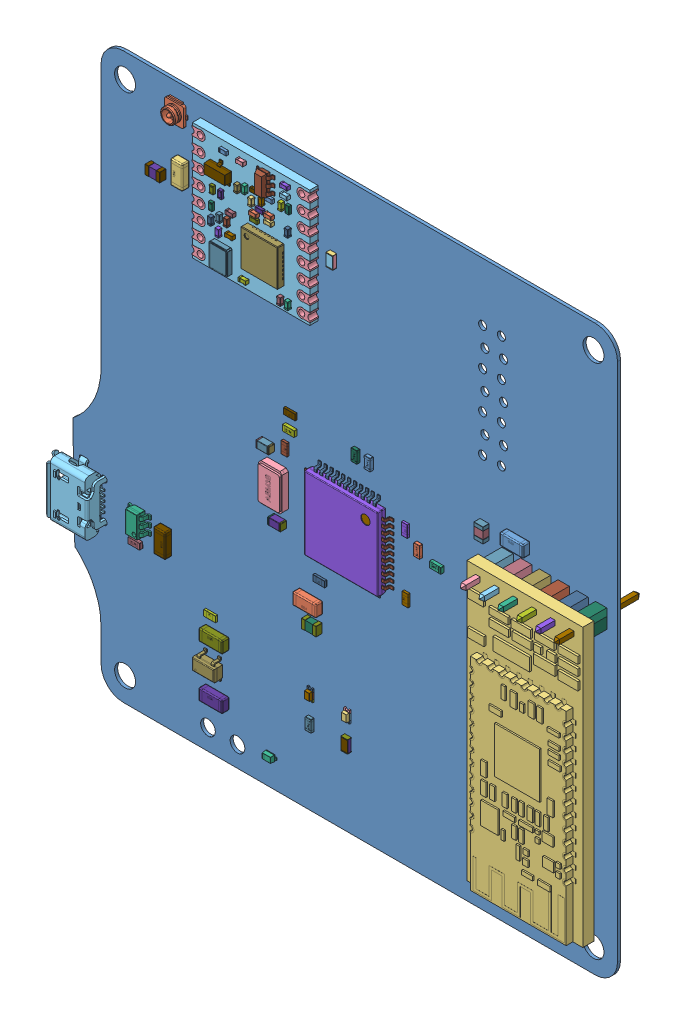
SolidWorks assembly Печатная плата Peggy Receiver, configuration Default. Lengths in mm. (continued)
Components (placement in the parent): (continued)
- Печатная плата Peggy Receiver(2)^Печатная плата Peggy Receiver-2: Печатная плата Peggy Receiver(2)^Печатная плата Peggy Receiver [Default] at origin size (75.31 78.06 11.44) (virtual) (continued)
  - DD1^Печатная плата Peggy Receiver(2)_Печатная плата Peggy Receiver-2: DD1^Печатная плата Peggy Receiver(2)_Печатная плата Peggy Receiver [Default] at origin size (16 15.9 2.23) (virtual) (continued)
    - User Library-RFM96W^DD1_Печатная плата Peggy Receiver(2)_Печатная плата Peggy Receiver-1: User Library-RFM96W^DD1_Печатная плата Peggy Receiver(2)_Печатная плата Peggy Receiver [Default] at (17.298 57.975 1.15) x (1 0 0) z (0 0 1) size (16 15.9 2.23) (virtual) (continued)
      - Designator8^User Library-RFM96W_DD1_Печатная плата Peggy Receiver(2)_Печатная плата Peggy Receiver-1: Designator8^User Library-RFM96W_DD1_Печатная плата Peggy Receiver(2)_Печатная плата Peggy Receiver [Default] at origin size (1 0.5 0.5) (virtual)
        - Cap0402^Designator8_User Library-RFM96W_DD1_Печатная плата Peggy Receiver(2)_Печатная плата Peggy Receiver-1: Cap0402^Designator8_User Library-RFM96W_DD1_Печатная плата Peggy Receiver(2)_Печатная плата Peggy Receiver [Default] at (5.4 5.45 0) x (1 0 0) z (0 -1 0) size (1 0.5 0.5) (virtual)
      - Designator9^User Library-RFM96W_DD1_Печатная плата Peggy Receiver(2)_Печатная плата Peggy Receiver-1: Designator9^User Library-RFM96W_DD1_Печатная плата Peggy Receiver(2)_Печатная плата Peggy Receiver [Default] at origin size (0.5 1 0.5) (virtual)
        - Cap0402^Designator9_User Library-RFM96W_DD1_Печатная плата Peggy Receiver(2)_Печатная плата Peggy Receiver-1: Cap0402^Designator9_User Library-RFM96W_DD1_Печатная плата Peggy Receiver(2)_Печатная плата Peggy Receiver [Default] at (2.8 5.98 0) x (0 -1 0) z (-1 0 0) size (1 0.5 0.5) (virtual)
      - Designator10^User Library-RFM96W_DD1_Печатная плата Peggy Receiver(2)_Печатная плата Peggy Receiver-1: Designator10^User Library-RFM96W_DD1_Печатная плата Peggy Receiver(2)_Печатная плата Peggy Receiver [Default] at origin size (0.5 1 0.5) (virtual)
        - Cap0402^Designator10_User Library-RFM96W_DD1_Печатная плата Peggy Receiver(2)_Печатная плата Peggy Receiver-1: Cap0402^Designator10_User Library-RFM96W_DD1_Печатная плата Peggy Receiver(2)_Печатная плата Peggy Receiver [Default] at (4.953 6.858 0) x (0 -1 0) z (-1 0 0) size (1 0.5 0.5) (virtual)
      - Designator11^User Library-RFM96W_DD1_Печатная плата Peggy Receiver(2)_Печатная плата Peggy Receiver-1: Designator11^User Library-RFM96W_DD1_Печатная плата Peggy Receiver(2)_Печатная плата Peggy Receiver [Default] at origin size (0.5 1 0.5) (virtual)
        - Cap0402^Designator11_User Library-RFM96W_DD1_Печатная плата Peggy Receiver(2)_Печатная плата Peggy Receiver-1: Cap0402^Designator11_User Library-RFM96W_DD1_Печатная плата Peggy Receiver(2)_Печатная плата Peggy Receiver [Default] at (6.35 11.557 0) x (0 1 0) z (1 0 0) size (1 0.5 0.5) (virtual)
      - Designator12^User Library-RFM96W_DD1_Печатная плата Peggy Receiver(2)_Печатная плата Peggy Receiver-1: Designator12^User Library-RFM96W_DD1_Печатная плата Peggy Receiver(2)_Печатная плата Peggy Receiver [Default] at origin size (1 0.5 0.5) (virtual)
        - Cap0402^Designator12_User Library-RFM96W_DD1_Печатная плата Peggy Receiver(2)_Печатная плата Peggy Receiver-1: Cap0402^Designator12_User Library-RFM96W_DD1_Печатная плата Peggy Receiver(2)_Печатная плата Peggy Receiver [Default] at (5.461 8.128 0) x (1 0 0) z (0 -1 0) size (1 0.5 0.5) (virtual)
      - Designator13^User Library-RFM96W_DD1_Печатная плата Peggy Receiver(2)_Печатная плата Peggy Receiver-1: Designator13^User Library-RFM96W_DD1_Печатная плата Peggy Receiver(2)_Печатная плата Peggy Receiver [Default] at origin size (0.5 1 0.5) (virtual)
        - Cap0402^Designator13_User Library-RFM96W_DD1_Печатная плата Peggy Receiver(2)_Печатная плата Peggy Receiver-1: Cap0402^Designator13_User Library-RFM96W_DD1_Печатная плата Peggy Receiver(2)_Печатная плата Peggy Receiver [Default] at (3.937 6.858 0) x (0 1 0) z (1 0 0) size (1 0.5 0.5) (virtual)
      - Designator15^User Library-RFM96W_DD1_Печатная плата Peggy Receiver(2)_Печатная плата Peggy Receiver-1: Designator15^User Library-RFM96W_DD1_Печатная плата Peggy Receiver(2)_Печатная плата Peggy Receiver [Default] at origin size (0.52 1.02 0.37) (virtual)
        - SW3dPS-inductor_0402_white^Designator15_User Library-RFM96W_DD1_Печатная плата Peggy Receiver(2)_Печатная плата Peggy Receiver-1: SW3dPS-inductor_0402_white^Designator15_User Library-RFM96W_DD1_Печатная плата Peggy Receiver(2)_Печатная плата Peggy Receiver [Default] at (13.208 12.446 0) x (1 0 0) z (0 -1 0) size (0.52 0.37 1.02) (virtual)
      - Designator17^User Library-RFM96W_DD1_Печатная плата Peggy Receiver(2)_Печатная плата Peggy Receiver-1: Designator17^User Library-RFM96W_DD1_Печатная плата Peggy Receiver(2)_Печатная плата Peggy Receiver [Default] at origin size (1.02 0.52 0.37) (virtual)
        - SW3dPS-inductor_0402_white^Designator17_User Library-RFM96W_DD1_Печатная плата Peggy Receiver(2)_Печатная плата Peggy Receiver-1: SW3dPS-inductor_0402_white^Designator17_User Library-RFM96W_DD1_Печатная плата Peggy Receiver(2)_Печатная плата Peggy Receiver [Default] at (8.636 8.89 0) x (0 1 0) z (1 0 0) size (0.52 0.37 1.02) (virtual)
      - Designator18^User Library-RFM96W_DD1_Печатная плата Peggy Receiver(2)_Печатная плата Peggy Receiver-1: Designator18^User Library-RFM96W_DD1_Печатная плата Peggy Receiver(2)_Печатная плата Peggy Receiver [Default] at origin size (1.02 0.52 0.37) (virtual)
        - SW3dPS-inductor_0402_white^Designator18_User Library-RFM96W_DD1_Печатная плата Peggy Receiver(2)_Печатная плата Peggy Receiver-1: SW3dPS-inductor_0402_white^Designator18_User Library-RFM96W_DD1_Печатная плата Peggy Receiver(2)_Печатная плата Peggy Receiver [Default] at (9.398 10.414 0) x (0 1 0) z (1 0 0) size (0.52 0.37 1.02) (virtual)
      - Designator19^User Library-RFM96W_DD1_Печатная плата Peggy Receiver(2)_Печатная плата Peggy Receiver-1: Designator19^User Library-RFM96W_DD1_Печатная плата Peggy Receiver(2)_Печатная плата Peggy Receiver [Default] at origin size (1.02 0.52 0.37) (virtual)
        - SW3dPS-inductor_0402_white^Designator19_User Library-RFM96W_DD1_Печатная плата Peggy Receiver(2)_Печатная плата Peggy Receiver-1: SW3dPS-inductor_0402_white^Designator19_User Library-RFM96W_DD1_Печатная плата Peggy Receiver(2)_Печатная плата Peggy Receiver [Default] at (8.636 12.319 0) x (0 1 0) z (1 0 0) size (0.52 0.37 1.02) (virtual)
      - Designator20^User Library-RFM96W_DD1_Печатная плата Peggy Receiver(2)_Печатная плата Peggy Receiver-1: Designator20^User Library-RFM96W_DD1_Печатная плата Peggy Receiver(2)_Печатная плата Peggy Receiver [Default] at origin size (1.02 0.52 0.37) (virtual)
        - SW3dPS-inductor_0402_white^Designator20_User Library-RFM96W_DD1_Печатная плата Peggy Receiver(2)_Печатная плата Peggy Receiver-1: SW3dPS-inductor_0402_white^Designator20_User Library-RFM96W_DD1_Печатная плата Peggy Receiver(2)_Печатная плата Peggy Receiver [Default] at (10.668 12.319 0) x (0 1 0) z (1 0 0) size (0.52 0.37 1.02) (virtual)
      - Designator21^User Library-RFM96W_DD1_Печатная плата Peggy Receiver(2)_Печатная плата Peggy Receiver-1: Designator21^User Library-RFM96W_DD1_Печатная плата Peggy Receiver(2)_Печатная плата Peggy Receiver [Default] at origin size (1 0.5 0.5) (virtual)
        - Cap0402^Designator21_User Library-RFM96W_DD1_Печатная плата Peggy Receiver(2)_Печатная плата Peggy Receiver-1: Cap0402^Designator21_User Library-RFM96W_DD1_Печатная плата Peggy Receiver(2)_Печатная плата Peggy Receiver [Default] at (10.668 10.414 0) x (-1 0 0) z (0 1 0) size (1 0.5 0.5) (virtual)
      - Designator22^User Library-RFM96W_DD1_Печатная плата Peggy Receiver(2)_Печатная плата Peggy Receiver-1: Designator22^User Library-RFM96W_DD1_Печатная плата Peggy Receiver(2)_Печатная плата Peggy Receiver [Default] at origin size (0.5 1 0.5) (virtual)
        - Cap0402^Designator22_User Library-RFM96W_DD1_Печатная плата Peggy Receiver(2)_Печатная плата Peggy Receiver-1: Cap0402^Designator22_User Library-RFM96W_DD1_Печатная плата Peggy Receiver(2)_Печатная плата Peggy Receiver [Default] at (8.255 10.922 0) x (0 1 0) z (1 0 0) size (1 0.5 0.5) (virtual)
      - Designator23^User Library-RFM96W_DD1_Печатная плата Peggy Receiver(2)_Печатная плата Peggy Receiver-1: Designator23^User Library-RFM96W_DD1_Печатная плата Peggy Receiver(2)_Печатная плата Peggy Receiver [Default] at origin size (1 0.5 0.5) (virtual)
        - Cap0402^Designator23_User Library-RFM96W_DD1_Печатная плата Peggy Receiver(2)_Печатная плата Peggy Receiver-1: Cap0402^Designator23_User Library-RFM96W_DD1_Печатная плата Peggy Receiver(2)_Печатная плата Peggy Receiver [Default] at (6.858 14.859 0) x (-1 0 0) z (0 1 0) size (1 0.5 0.5) (virtual)
      - Designator24^User Library-RFM96W_DD1_Печатная плата Peggy Receiver(2)_Печатная плата Peggy Receiver-1: Designator24^User Library-RFM96W_DD1_Печатная плата Peggy Receiver(2)_Печатная плата Peggy Receiver [Default] at origin size (1 0.5 0.5) (virtual)
        - Cap0402^Designator24_User Library-RFM96W_DD1_Печатная плата Peggy Receiver(2)_Печатная плата Peggy Receiver-1: Cap0402^Designator24_User Library-RFM96W_DD1_Печатная плата Peggy Receiver(2)_Печатная плата Peggy Receiver [Default] at (12.827 13.843 0) x (-1 0 0) z (0 1 0) size (1 0.5 0.5) (virtual)
      - Designator25^User Library-RFM96W_DD1_Печатная плата Peggy Receiver(2)_Печатная плата Peggy Receiver-1: Designator25^User Library-RFM96W_DD1_Печатная плата Peggy Receiver(2)_Печатная плата Peggy Receiver [Default] at origin size (0.5 1 0.5) (virtual)
        - Cap0402^Designator25_User Library-RFM96W_DD1_Печатная плата Peggy Receiver(2)_Печатная плата Peggy Receiver-1: Cap0402^Designator25_User Library-RFM96W_DD1_Печатная плата Peggy Receiver(2)_Печатная плата Peggy Receiver [Default] at (7.366 11.938 0) x (0 -1 0) z (-1 0 0) size (1 0.5 0.5) (virtual)
      - Designator26^User Library-RFM96W_DD1_Печатная плата Peggy Receiver(2)_Печатная плата Peggy Receiver-1: Designator26^User Library-RFM96W_DD1_Печатная плата Peggy Receiver(2)_Печатная плата Peggy Receiver [Default] at origin size (0.5 1 0.5) (virtual)
        - Cap0402^Designator26_User Library-RFM96W_DD1_Печатная плата Peggy Receiver(2)_Печатная плата Peggy Receiver-1: Cap0402^Designator26_User Library-RFM96W_DD1_Печатная плата Peggy Receiver(2)_Печатная плата Peggy Receiver [Default] at (12.319 12.446 0) x (0 -1 0) z (-1 0 0) size (1 0.5 0.5) (virtual)
      - Designator27^User Library-RFM96W_DD1_Печатная плата Peggy Receiver(2)_Печатная плата Peggy Receiver-1: Designator27^User Library-RFM96W_DD1_Печатная плата Peggy Receiver(2)_Печатная плата Peggy Receiver [Default] at origin size (1 0.5 0.5) (virtual)
        - Cap0402^Designator27_User Library-RFM96W_DD1_Печатная плата Peggy Receiver(2)_Печатная плата Peggy Receiver-1: Cap0402^Designator27_User Library-RFM96W_DD1_Печатная плата Peggy Receiver(2)_Печатная плата Peggy Receiver [Default] at (12.827 14.986 0) x (-1 0 0) z (0 1 0) size (1 0.5 0.5) (virtual)
      - Designator28^User Library-RFM96W_DD1_Печатная плата Peggy Receiver(2)_Печатная плата Peggy Receiver-1: Designator28^User Library-RFM96W_DD1_Печатная плата Peggy Receiver(2)_Печатная плата Peggy Receiver [Default] at origin size (0.5 1 0.5) (virtual)
        - Cap0402^Designator28_User Library-RFM96W_DD1_Печатная плата Peggy Receiver(2)_Печатная плата Peggy Receiver-1: Cap0402^Designator28_User Library-RFM96W_DD1_Печатная плата Peggy Receiver(2)_Печатная плата Peggy Receiver [Default] at (9.652 11.684 0) x (0 -1 0) z (-1 0 0) size (1 0.5 0.5) (virtual)
      - Designator29^User Library-RFM96W_DD1_Печатная плата Peggy Receiver(2)_Печатная плата Peggy Receiver-1: Designator29^User Library-RFM96W_DD1_Печатная плата Peggy Receiver(2)_Печатная плата Peggy Receiver [Default] at origin size (0.5 1 0.5) (virtual)
        - Cap0402^Designator29_User Library-RFM96W_DD1_Печатная плата Peggy Receiver(2)_Печатная плата Peggy Receiver-1: Cap0402^Designator29_User Library-RFM96W_DD1_Печатная плата Peggy Receiver(2)_Печатная плата Peggy Receiver [Default] at (13.208 9.779 0) x (0 -1 0) z (-1 0 0) size (1 0.5 0.5) (virtual)
      - Designator27_2^User Library-RFM96W_DD1_Печатная плата Peggy Receiver(2)_Печатная плата Peggy Receiver-1: Designator27_2^User Library-RFM96W_DD1_Печатная плата Peggy Receiver(2)_Печатная плата Peggy Receiver [Default] at origin size (2.43 2.79 1.09) (virtual)
        - SW3dPS-SOT-23-6^Designator27_2_User Library-RFM96W_DD1_Печатная плата Peggy Receiver(2)_Печатная плата Peggy Receiver-1: SW3dPS-SOT-23-6^Designator27_2_User Library-RFM96W_DD1_Печатная плата Peggy Receiver(2)_Печатная плата Peggy Receiver [Default] at (9.0742 15.0495 0) x (0 -1 0) z (0 0 1) size (2.79 2.43 1.09) (virtual)
      - Designator2^User Library-RFM96W_DD1_Печатная плата Peggy Receiver(2)_Печатная плата Peggy Receiver-1: Designator2^User Library-RFM96W_DD1_Печатная плата Peggy Receiver(2)_Печатная плата Peggy Receiver [Default] at origin size (5.04 5.04 0.9) (virtual)
        - QFN28^Designator2_User Library-RFM96W_DD1_Печатная плата Peggy Receiver(2)_Печатная плата Peggy Receiver-1: QFN28^Designator2_User Library-RFM96W_DD1_Печатная плата Peggy Receiver(2)_Печатная плата Peggy Receiver [Default] at (9.97 5.42 0) x (0 -1 0) z (-1 0 0) size (5.04 0.9 5.04) (virtual)
      - Designator5^User Library-RFM96W_DD1_Печатная плата Peggy Receiver(2)_Печатная плата Peggy Receiver-1: Designator5^User Library-RFM96W_DD1_Печатная плата Peggy Receiver(2)_Печатная плата Peggy Receiver [Default] at origin size (0.5 1 0.5) (virtual)
        - Cap0402^Designator5_User Library-RFM96W_DD1_Печатная плата Peggy Receiver(2)_Печатная плата Peggy Receiver-1: Cap0402^Designator5_User Library-RFM96W_DD1_Печатная плата Peggy Receiver(2)_Печатная плата Peggy Receiver [Default] at (12.192 1.27 0) x (0 -1 0) z (-1 0 0) size (1 0.5 0.5) (virtual)
      - Designator1^User Library-RFM96W_DD1_Печатная плата Peggy Receiver(2)_Печатная плата Peggy Receiver-1: Designator1^User Library-RFM96W_DD1_Печатная плата Peggy Receiver(2)_Печатная плата Peggy Receiver [Default] at origin size (2.5 3.2 0.7) (virtual)
        - TXC_7M^Designator1_User Library-RFM96W_DD1_Печатная плата Peggy Receiver(2)_Печатная плата Peggy Receiver-1: TXC_7M^Designator1_User Library-RFM96W_DD1_Печатная плата Peggy Receiver(2)_Печатная плата Peggy Receiver [Default] at (4.1911 2.286 0) x (0 1 0) z (1 0 0) size (3.2 0.7 2.5) (virtual)
      - Open CASCADE STEP translator 6.5 1.29^User Library-RFM96W_DD1_Печатная плата Peggy Receiver(2)_Печатная плата Peggy Receiver-1: Open CASCADE STEP translator 6.5 1.29^User Library-RFM96W_DD1_Печатная плата Peggy Receiver(2)_Печатная плата Peggy Receiver [Default] at origin size (0.5 1 0.35) (virtual)
        - Res0402^Open CASCADE STEP translator 6.5 1.29_User Library-RFM96W_DD1_Печатная плата Peggy Receiver(2)_Печатная плата Peggy Receiver-1: Res0402^Open CASCADE STEP translator 6.5 1.29_User Library-RFM96W_DD1_Печатная плата Peggy Receiver(2)_Печатная плата Peggy Receiver [Default] at (2.794 7.62 0) x (0 1 0) z (1 0 0) size (1 0.35 0.5) (virtual)
      - 1^User Library-RFM96W_DD1_Печатная плата Peggy Receiver(2)_Печатная плата Peggy Receiver-1: 1^User Library-RFM96W_DD1_Печатная плата Peggy Receiver(2)_Печатная плата Peggy Receiver [Default] at origin size (0.5 1 0.35) (virtual)
        - Res0402^1_User Library-RFM96W_DD1_Печатная плата Peggy Receiver(2)_Печатная плата Peggy Receiver-1: Res0402^1_User Library-RFM96W_DD1_Печатная плата Peggy Receiver(2)_Печатная плата Peggy Receiver [Default] at (2.921 9.652 0) x (0 1 0) z (1 0 0) size (1 0.35 0.5) (virtual)
      - 2^User Library-RFM96W_DD1_Печатная плата Peggy Receiver(2)_Печатная плата Peggy Receiver-1: 2^User Library-RFM96W_DD1_Печатная плата Peggy Receiver(2)_Печатная плата Peggy Receiver [Default] at origin size (0.5 1 0.35) (virtual)
        - Res0402^2_User Library-RFM96W_DD1_Печатная плата Peggy Receiver(2)_Печатная плата Peggy Receiver-1: Res0402^2_User Library-RFM96W_DD1_Печатная плата Peggy Receiver(2)_Печатная плата Peggy Receiver [Default] at (4.064 9.652 0) x (0 1 0) z (1 0 0) size (1 0.35 0.5) (virtual)
      - Open CASCADE STEP translator 6.5 1.32^User Library-RFM96W_DD1_Печатная плата Peggy Receiver(2)_Печатная плата Peggy Receiver-1: Open CASCADE STEP translator 6.5 1.32^User Library-RFM96W_DD1_Печатная плата Peggy Receiver(2)_Печатная плата Peggy Receiver [Default] at origin size (3.03 2.48 1.12) (virtual)
        - User_Library-3-lead_sot23-3^Open CASCADE STEP translator 6.5 1.32_User Library-RFM96W_DD1_Печатная плата Peggy Receiver(2)_Печатная плата Peggy Receiver-1: User_Library-3-lead_sot23-3^Open CASCADE STEP translator 6.5 1.32_User Library-RFM96W_DD1_Печатная плата Peggy Receiver(2)_Печатная плата Peggy Receiver [Default] at (3.9981 12.3031 0.35) x (1 0 0) z (0 -1 0) size (3.03 1.12 2.48) (virtual)
      - 3^User Library-RFM96W_DD1_Печатная плата Peggy Receiver(2)_Печатная плата Peggy Receiver-1: 3^User Library-RFM96W_DD1_Печатная плата Peggy Receiver(2)_Печатная плата Peggy Receiver [Default] at origin size (1 0.5 0.35) (virtual)
        - Res0402^3_User Library-RFM96W_DD1_Печатная плата Peggy Receiver(2)_Печатная плата Peggy Receiver-1: Res0402^3_User Library-RFM96W_DD1_Печатная плата Peggy Receiver(2)_Печатная плата Peggy Receiver [Default] at (4.445 14.859 0) x (-1 0 0) z (0 1 0) size (1 0.35 0.5) (virtual)
      - Designator31^User Library-RFM96W_DD1_Печатная плата Peggy Receiver(2)_Печатная плата Peggy Receiver-1: Designator31^User Library-RFM96W_DD1_Печатная плата Peggy Receiver(2)_Печатная плата Peggy Receiver [Default] at origin size (1 0.5 0.5) (virtual)
        - Cap0402^Designator31_User Library-RFM96W_DD1_Печатная плата Peggy Receiver(2)_Печатная плата Peggy Receiver-1: Cap0402^Designator31_User Library-RFM96W_DD1_Печатная плата Peggy Receiver(2)_Печатная плата Peggy Receiver [Default] at (8.636 9.652 0) x (-1 0 0) z (0 1 0) size (1 0.5 0.5) (virtual)
      - Designator32^User Library-RFM96W_DD1_Печатная плата Peggy Receiver(2)_Печатная плата Peggy Receiver-1: Designator32^User Library-RFM96W_DD1_Печатная плата Peggy Receiver(2)_Печатная плата Peggy Receiver [Default] at origin size (1 0.5 0.5) (virtual)
        - Cap0402^Designator32_User Library-RFM96W_DD1_Печатная плата Peggy Receiver(2)_Печатная плата Peggy Receiver-1: Cap0402^Designator32_User Library-RFM96W_DD1_Печатная плата Peggy Receiver(2)_Печатная плата Peggy Receiver [Default] at (10.668 9.652 0) x (-1 0 0) z (0 1 0) size (1 0.5 0.5) (virtual)
      - Free-Models^User Library-RFM96W_DD1_Печатная плата Peggy Receiver(2)_Печатная плата Peggy Receiver-1: Free-Models^User Library-RFM96W_DD1_Печатная плата Peggy Receiver(2)_Печатная плата Peggy Receiver [Default] at origin size (16 15.3 1.16) (virtual)
        - Goldcontact^Free-Models_User Library-RFM96W_DD1_Печатная плата Peggy Receiver(2)_Печатная плата Peggy Receiver-1: Goldcontact^Free-Models_User Library-RFM96W_DD1_Печатная плата Peggy Receiver(2)_Печатная плата Peggy Receiver [Default] at (0.56 1 -1.14) x (-1 0 0) z (0 1 0) size (1.77 1.16 1.3) (virtual)
        - Goldcontact^Free-Models_User Library-RFM96W_DD1_Печатная плата Peggy Receiver(2)_Печатная плата Peggy Receiver-2: Goldcontact^Free-Models_User Library-RFM96W_DD1_Печатная плата Peggy Receiver(2)_Печатная плата Peggy Receiver [Default] at (0.56 3 -1.14) x (-1 0 0) z (0 1 0) size (1.77 1.16 1.3) (virtual)
        - Goldcontact^Free-Models_User Library-RFM96W_DD1_Печатная плата Peggy Receiver(2)_Печатная плата Peggy Receiver-3: Goldcontact^Free-Models_User Library-RFM96W_DD1_Печатная плата Peggy Receiver(2)_Печатная плата Peggy Receiver [Default] at (0.56 5 -1.14) x (-1 0 0) z (0 1 0) size (1.77 1.16 1.3) (virtual)
        - Goldcontact^Free-Models_User Library-RFM96W_DD1_Печатная плата Peggy Receiver(2)_Печатная плата Peggy Receiver-4: Goldcontact^Free-Models_User Library-RFM96W_DD1_Печатная плата Peggy Receiver(2)_Печатная плата Peggy Receiver [Default] at (0.56 7 -1.14) x (-1 0 0) z (0 1 0) size (1.77 1.16 1.3) (virtual)
        - Goldcontact^Free-Models_User Library-RFM96W_DD1_Печатная плата Peggy Receiver(2)_Печатная плата Peggy Receiver-5: Goldcontact^Free-Models_User Library-RFM96W_DD1_Печатная плата Peggy Receiver(2)_Печатная плата Peggy Receiver [Default] at (0.56 9 -1.14) x (-1 0 0) z (0 1 0) size (1.77 1.16 1.3) (virtual)
        - Goldcontact^Free-Models_User Library-RFM96W_DD1_Печатная плата Peggy Receiver(2)_Печатная плата Peggy Receiver-6: Goldcontact^Free-Models_User Library-RFM96W_DD1_Печатная плата Peggy Receiver(2)_Печатная плата Peggy Receiver [Default] at (0.56 11 -1.14) x (-1 0 0) z (0 1 0) size (1.77 1.16 1.3) (virtual)
        - Goldcontact^Free-Models_User Library-RFM96W_DD1_Печатная плата Peggy Receiver(2)_Печатная плата Peggy Receiver-7: Goldcontact^Free-Models_User Library-RFM96W_DD1_Печатная плата Peggy Receiver(2)_Печатная плата Peggy Receiver [Default] at (0.56 13 -1.14) x (-1 0 0) z (0 1 0) size (1.77 1.16 1.3) (virtual)
        - Goldcontact^Free-Models_User Library-RFM96W_DD1_Печатная плата Peggy Receiver(2)_Печатная плата Peggy Receiver-8: Goldcontact^Free-Models_User Library-RFM96W_DD1_Печатная плата Peggy Receiver(2)_Печатная плата Peggy Receiver [Default] at (0.56 15 -1.14) x (-1 0 0) z (0 1 0) size (1.77 1.16 1.3) (virtual)
        - Goldcontact^Free-Models_User Library-RFM96W_DD1_Печатная плата Peggy Receiver(2)_Печатная плата Peggy Receiver-9: Goldcontact^Free-Models_User Library-RFM96W_DD1_Печатная плата Peggy Receiver(2)_Печатная плата Peggy Receiver [Default] at (15.442 15 -1.14) x (1 0 0) z (0 -1 0) size (1.77 1.16 1.3) (virtual)
        - Goldcontact^Free-Models_User Library-RFM96W_DD1_Печатная плата Peggy Receiver(2)_Печатная плата Peggy Receiver-10: Goldcontact^Free-Models_User Library-RFM96W_DD1_Печатная плата Peggy Receiver(2)_Печатная плата Peggy Receiver [Default] at (15.442 13 -1.14) x (1 0 0) z (0 -1 0) size (1.77 1.16 1.3) (virtual)
        - Goldcontact^Free-Models_User Library-RFM96W_DD1_Печатная плата Peggy Receiver(2)_Печатная плата Peggy Receiver-11: Goldcontact^Free-Models_User Library-RFM96W_DD1_Печатная плата Peggy Receiver(2)_Печатная плата Peggy Receiver [Default] at (15.442 11 -1.14) x (1 0 0) z (0 -1 0) size (1.77 1.16 1.3) (virtual)
        - Goldcontact^Free-Models_User Library-RFM96W_DD1_Печатная плата Peggy Receiver(2)_Печатная плата Peggy Receiver-12: Goldcontact^Free-Models_User Library-RFM96W_DD1_Печатная плата Peggy Receiver(2)_Печатная плата Peggy Receiver [Default] at (15.442 9 -1.14) x (1 0 0) z (0 -1 0) size (1.77 1.16 1.3) (virtual)
        - Goldcontact^Free-Models_User Library-RFM96W_DD1_Печатная плата Peggy Receiver(2)_Печатная плата Peggy Receiver-13: Goldcontact^Free-Models_User Library-RFM96W_DD1_Печатная плата Peggy Receiver(2)_Печатная плата Peggy Receiver [Default] at (15.442 7 -1.14) x (1 0 0) z (0 -1 0) size (1.77 1.16 1.3) (virtual)
        - Goldcontact^Free-Models_User Library-RFM96W_DD1_Печатная плата Peggy Receiver(2)_Печатная плата Peggy Receiver-14: Goldcontact^Free-Models_User Library-RFM96W_DD1_Печатная плата Peggy Receiver(2)_Печатная плата Peggy Receiver [Default] at (15.442 5 -1.14) x (1 0 0) z (0 -1 0) size (1.77 1.16 1.3) (virtual)
        - Goldcontact^Free-Models_User Library-RFM96W_DD1_Печатная плата Peggy Receiver(2)_Печатная плата Peggy Receiver-15: Goldcontact^Free-Models_User Library-RFM96W_DD1_Печатная плата Peggy Receiver(2)_Печатная плата Peggy Receiver [Default] at (15.442 3 -1.14) x (1 0 0) z (0 -1 0) size (1.77 1.16 1.3) (virtual)
        - Goldcontact^Free-Models_User Library-RFM96W_DD1_Печатная плата Peggy Receiver(2)_Печатная плата Peggy Receiver-16: Goldcontact^Free-Models_User Library-RFM96W_DD1_Печатная плата Peggy Receiver(2)_Печатная плата Peggy Receiver [Default] at (15.442 1 -1.14) x (1 0 0) z (0 -1 0) size (1.77 1.16 1.3) (virtual)
      - Board-4^User Library-RFM96W_DD1_Печатная плата Peggy Receiver(2)_Печатная плата Peggy Receiver-1: Board-4^User Library-RFM96W_DD1_Печатная плата Peggy Receiver(2)_Печатная плата Peggy Receiver [Default] at (0 0 -1.1204) size (15.9 15.9 1.12) (virtual)
  - D2^Печатная плата Peggy Receiver(2)_Печатная плата Peggy Receiver-2: D2^Печатная плата Peggy Receiver(2)_Печатная плата Peggy Receiver [Default] at origin size (3 3 1.3) (virtual)
    - SOT23-5-1^D2_Печатная плата Peggy Receiver(2)_Печатная плата Peggy Receiver-1: SOT23-5-1^D2_Печатная плата Peggy Receiver(2)_Печатная плата Peggy Receiver [Default] at (9.1731 22.6912 0) x (-1 0 0) z (0 0 1) size (3 3 1.3) (virtual)
  - C14^Печатная плата Peggy Receiver(2)_Печатная плата Peggy Receiver-2: C14^Печатная плата Peggy Receiver(2)_Печатная плата Peggy Receiver [Default] at origin size (1.6 0.8 0.3) (virtual)
    - SW3dPS-0603 SMD Capacitor^C14_Печатная плата Peggy Receiver(2)_Печатная плата Peggy Receiver-1: SW3dPS-0603 SMD Capacitor^C14_Печатная плата Peggy Receiver(2)_Печатная плата Peggy Receiver [Default] at (18.8091 16.273 0) x (1 0 0) z (0 -1 0) size (1.6 0.3 0.8) (virtual)
  - C10^Печатная плата Peggy Receiver(2)_Печатная плата Peggy Receiver-2: C10^Печатная плата Peggy Receiver(2)_Печатная плата Peggy Receiver [Default] at origin size (0.8 1.6 0.3) (virtual)
    - SW3dPS-0603 SMD Capacitor^C10_Печатная плата Peggy Receiver(2)_Печатная плата Peggy Receiver-1: SW3dPS-0603 SMD Capacitor^C10_Печатная плата Peggy Receiver(2)_Печатная плата Peggy Receiver [Default] at (45.2091 39.5728 0) x (0 -1 0) z (-1 0 0) size (1.6 0.3 0.8) (virtual)
  - C9^Печатная плата Peggy Receiver(2)_Печатная плата Peggy Receiver-2: C9^Печатная плата Peggy Receiver(2)_Печатная плата Peggy Receiver [Default] at origin size (0.8 1.6 0.3) (virtual)
    - SW3dPS-0603 SMD Capacitor^C9_Печатная плата Peggy Receiver(2)_Печатная плата Peggy Receiver-1: SW3dPS-0603 SMD Capacitor^C9_Печатная плата Peggy Receiver(2)_Печатная плата Peggy Receiver [Default] at (45.3089 31.473 0) x (0 1 0) z (1 0 0) size (1.6 0.3 0.8) (virtual)
  - C8^Печатная плата Peggy Receiver(2)_Печатная плата Peggy Receiver-2: C8^Печатная плата Peggy Receiver(2)_Печатная плата Peggy Receiver [Default] at origin size (1.6 0.8 0.3) (virtual)
    - SW3dPS-0603 SMD Capacitor^C8_Печатная плата Peggy Receiver(2)_Печатная плата Peggy Receiver-1: SW3dPS-0603 SMD Capacitor^C8_Печатная плата Peggy Receiver(2)_Печатная плата Peggy Receiver [Default] at (33.6089 27.7728 0) x (-1 0 0) z (0 1 0) size (1.6 0.3 0.8) (virtual)
  - C7^Печатная плата Peggy Receiver(2)_Печатная плата Peggy Receiver-2: C7^Печатная плата Peggy Receiver(2)_Печатная плата Peggy Receiver [Default] at origin size (0.8 1.6 0.3) (virtual)
    - SW3dPS-0603 SMD Capacitor^C7_Печатная плата Peggy Receiver(2)_Печатная плата Peggy Receiver-1: SW3dPS-0603 SMD Capacitor^C7_Печатная плата Peggy Receiver(2)_Печатная плата Peggy Receiver [Default] at (28.9091 40.9728 0) x (0 -1 0) z (-1 0 0) size (1.6 0.3 0.8) (virtual)
  - C3^Печатная плата Peggy Receiver(2)_Печатная плата Peggy Receiver-2: C3^Печатная плата Peggy Receiver(2)_Печатная плата Peggy Receiver [Default] at origin size (1.75 0.95 0.87) (virtual)
    - 6665910208^C3_Печатная плата Peggy Receiver(2)_Печатная плата Peggy Receiver-1: 6665910208^C3_Печатная плата Peggy Receiver(2)_Печатная плата Peggy Receiver [Default] at (26.5 40.2 0) x (-1 0 0) z (0 0 1) size (1.75 0.95 0.87) (virtual)
      - Terminal-2^6665910208_C3_Печатная плата Peggy Receiver(2)_Печатная плата Peggy Receiver-1: Terminal-2^6665910208_C3_Печатная плата Peggy Receiver(2)_Печатная плата Peggy Receiver [Default] at (-0.875 -0.475 0) size (1.75 0.95 0.87) (virtual)
        - Open CASCADE STEP translator 6.8 127.1.1^Terminal-2_6665910208_C3_Печатная плата Peggy Receiver(2)_Печатная плата Peggy Receiver-1: Open CASCADE STEP translator 6.8 127.1.1^Terminal-2_6665910208_C3_Печатная плата Peggy Receiver(2)_Печатная плата Peggy Receiver [Default] at origin size (0.2 0.95 0.87) (virtual)
        - Open CASCADE STEP translator 6.8 127.1.2^Terminal-2_6665910208_C3_Печатная плата Peggy Receiver(2)_Печатная плата Peggy Receiver-1: Open CASCADE STEP translator 6.8 127.1.2^Terminal-2_6665910208_C3_Печатная плата Peggy Receiver(2)_Печатная плата Peggy Receiver [Default] at origin size (0.2 0.95 0.87) (virtual)
      - Mid_Body-5^6665910208_C3_Печатная плата Peggy Receiver(2)_Печатная плата Peggy Receiver-1: Mid_Body-5^6665910208_C3_Печатная плата Peggy Receiver(2)_Печатная плата Peggy Receiver [Default] at (-0.875 -0.475 0) size (1.35 0.95 0.87) (virtual)
        - Open CASCADE STEP translator 6.8 127.2.1^Mid_Body-5_6665910208_C3_Печатная плата Peggy Receiver(2)_Печатная плата Peggy Receiver-1: Open CASCADE STEP translator 6.8 127.2.1^Mid_Body-5_6665910208_C3_Печатная плата Peggy Receiver(2)_Печатная плата Peggy Receiver [Default] at origin size (1.35 0.95 0.87) (virtual)
  - C2^Печатная плата Peggy Receiver(2)_Печатная плата Peggy Receiver-2: C2^Печатная плата Peggy Receiver(2)_Печатная плата Peggy Receiver [Default] at origin size (1.75 0.95 0.87) (virtual)
    - 6665910368^C2_Печатная плата Peggy Receiver(2)_Печатная плата Peggy Receiver-1: 6665910368^C2_Печатная плата Peggy Receiver(2)_Печатная плата Peggy Receiver [Default] at (28.109 31.9729 0) x (1 0 0) z (0 0 1) size (1.75 0.95 0.87) (virtual)
      - Terminal-3^6665910368_C2_Печатная плата Peggy Receiver(2)_Печатная плата Peggy Receiver-1: Terminal-3^6665910368_C2_Печатная плата Peggy Receiver(2)_Печатная плата Peggy Receiver [Default] at (-0.875 -0.475 0) size (1.75 0.95 0.87) (virtual)
        - Open CASCADE STEP translator 6.8 127.1.1-6^Terminal-3_6665910368_C2_Печатная плата Peggy Receiver(2)_Печатная плата Peggy Receiver-1: Open CASCADE STEP translator 6.8 127.1.1-6^Terminal-3_6665910368_C2_Печатная плата Peggy Receiver(2)_Печатная плата Peggy Receiver [Default] at origin size (0.2 0.95 0.87) (virtual)
        - Open CASCADE STEP translator 6.8 127.1.2-7^Terminal-3_6665910368_C2_Печатная плата Peggy Receiver(2)_Печатная плата Peggy Receiver-1: Open CASCADE STEP translator 6.8 127.1.2-7^Terminal-3_6665910368_C2_Печатная плата Peggy Receiver(2)_Печатная плата Peggy Receiver [Default] at origin size (0.2 0.95 0.87) (virtual)
      - Mid_Body-1-8^6665910368_C2_Печатная плата Peggy Receiver(2)_Печатная плата Peggy Receiver-1: Mid_Body-1-8^6665910368_C2_Печатная плата Peggy Receiver(2)_Печатная плата Peggy Receiver [Default] at (-0.875 -0.475 0) size (1.35 0.95 0.87) (virtual)
        - Open CASCADE STEP translator 6.8 127.2.1-9^Mid_Body-1-8_6665910368_C2_Печатная плата Peggy Receiver(2)_Печатная плата Peggy Receiver-1: Open CASCADE STEP translator 6.8 127.2.1-9^Mid_Body-1-8_6665910368_C2_Печатная плата Peggy Receiver(2)_Печатная плата Peggy Receiver [Default] at origin size (1.35 0.95 0.87) (virtual)
  - C1^Печатная плата Peggy Receiver(2)_Печатная плата Peggy Receiver-2: C1^Печатная плата Peggy Receiver(2)_Печатная плата Peggy Receiver [Default] at origin size (1.6 0.8 0.3) (virtual)
    - SW3dPS-0603 SMD Capacitor^C1_Печатная плата Peggy Receiver(2)_Печатная плата Peggy Receiver-1: SW3dPS-0603 SMD Capacitor^C1_Печатная плата Peggy Receiver(2)_Печатная плата Peggy Receiver [Default] at (29.6089 45.3728 0) x (-1 0 0) z (0 1 0) size (1.6 0.3 0.8) (virtual)
